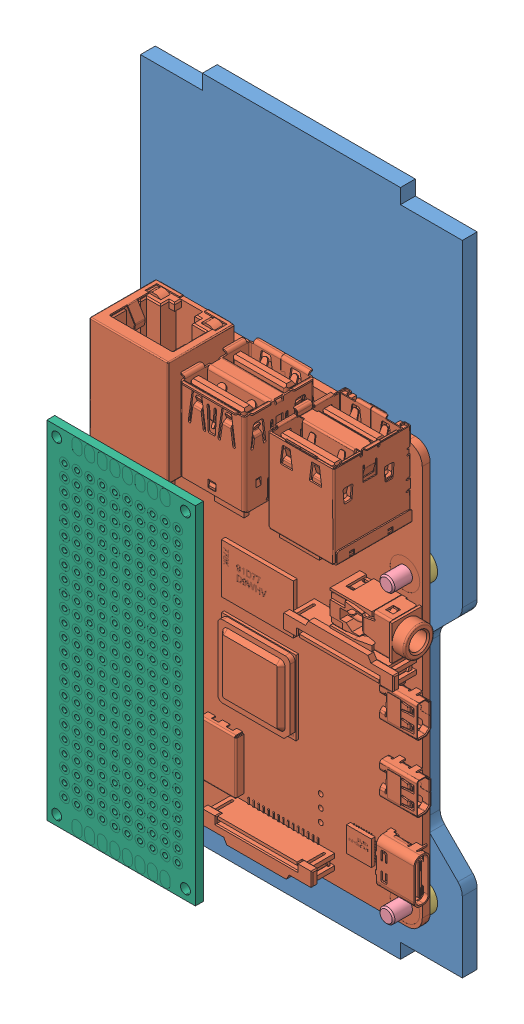
SolidWorks assembly ASM-level-raspberry-pi, configuration По умолчанию. Lengths in mm.
Overall size (65 135 24.74).
13 component instances, 6 part files, 17 mates.
Components (placement in the parent):
- level-2-1: level-2 [По умолчанию] at origin size (65 135 3)
- Raspberry Pi 4 Model B-1: Raspberry Pi 4 Model B [По умолчанию] at (0 -15 5.79) x (0 1 0) z (1 0 0) size (88.99 19.91 58.4)
- 3-6-3-1: 3-6-3 [По умолчанию] at (-24.5 -54 3) size (6 6 2)
- 3-6-3-2: 3-6-3 [По умолчанию] at (-24.5 4 3) size (6 6 2)
- 3-6-3-3: 3-6-3 [По умолчанию] at (24.5 4 3) size (6 6 2)
- 3-6-3-4: 3-6-3 [По умолчанию] at (24.5 -54 3) x (0.98212 -0.188257 0) z (0 0 1) size (6 6 2)
- socket countersunk head screw_iso-1: socket countersunk head screw_iso [ISO 10642 - M3 x 10 - 10N] at (24.5 -54 0.39) x (0 0 1) z (-0.999977 -0.006797 0) size (10 5.54 5.54)
- socket countersunk head screw_iso-2: socket countersunk head screw_iso [ISO 10642 - M3 x 10 - 10N] at (24.5 4 0.39) x (0 0 1) z (-0.999917 -0.012873 0) size (10 5.54 5.54)
- socket countersunk head screw_iso-3: socket countersunk head screw_iso [ISO 10642 - M3 x 10 - 10N] at (-24.5 4 0.39) x (0 0 1) z (-0.999928 -0.012001 0) size (10 5.54 5.54)
- socket countersunk head screw_iso-4: socket countersunk head screw_iso [ISO 10642 - M3 x 10 - 10N] at (-24.5 -54 0.39) x (0 0 1) z (-1 -0.000767 0) size (10 5.54 5.54)
- ASM-shild-raspberry-1: ASM-shild-raspberry [По умолчанию] at (-22.18 0.88 25.14) x (1 0 0) z (0 1 0) size (30 10.65 70)
  - 40 pin connector header smt v3.step-1: 40 pin connector header smt v3.step [По умолчанию] at origin size (5.18 10.05 51.4)
  - Breadboard 30 х 70 mm.step-1: Breadboard 30 х 70 mm.step [По умолчанию] at (7.5097 0.4 -23.0097) size (30 1.65 70)
Mates (geometry in assembly coordinates):
- Концентричный1: concentric anti-aligned: cylinder of level-2-1 through (-24.5 -54 -7) axis (0 0 1) radius 1.75; cylinder of 3-6-3-1 through (-24.5 -54 5) axis (0 0 -1) radius 1.75
- Концентричный2: concentric anti-aligned: cylinder of level-2-1 through (-24.5 4 -7) axis (0 0 1) radius 1.75; cylinder of 3-6-3-2 through (-24.5 4 5) axis (0 0 -1) radius 1.75
- Концентричный3: concentric anti-aligned: cylinder of level-2-1 through (24.5 4 -7) axis (0 0 1) radius 1.75; cylinder of 3-6-3-3 through (24.5 4 5) axis (0 0 -1) radius 1.75
- Концентричный4: concentric anti-aligned: cylinder of level-2-1 through (24.5 -54 -7) axis (0 0 1) radius 1.75; cylinder of 3-6-3-4 through (24.5 -54 5) axis (0 0 -1) radius 1.75
- Совпадение1: coincident aligned: plane of 3-6-3-1 through (-24.5 -54 5) normal (0 0 1); plane of 3-6-3-4 through (24.5 -54 5) normal (0 0 1)
- Совпадение2: coincident aligned: plane of 3-6-3-2 through (-24.5 4 5) normal (0 0 1); plane of 3-6-3-3 through (24.5 4 5) normal (0 0 1)
- Совпадение3: coincident aligned: plane of 3-6-3-3 through (24.5 4 5) normal (0 0 1); plane of 3-6-3-4 through (24.5 -54 5) normal (0 0 1)
- Совпадение4: coincident anti-aligned: plane of level-2-1 through (0 0 3) normal (0 0 1); plane of 3-6-3-4 through (24.5 -54 3) normal (0 0 -1)
- Концентричный5: concentric anti-aligned: cylinder of Raspberry Pi 4 Model B-1 through (24.5 -54 6.59) axis (0 0 1) radius 1.35; cylinder of 3-6-3-4 through (24.5 -54 5) axis (0 0 -1) radius 1.75
- Совпадение5: coincident anti-aligned: plane of Raspberry Pi 4 Model B-1 through (24.5 -54 5) normal (0 0 -1); plane of 3-6-3-4 through (24.5 -54 5) normal (0 0 1)
- Совпадение6: coincident aligned: cone of level-2-1 through (24.5 -54 0) axis (0 0 1); cone of socket countersunk head screw_iso-1 through (24.5 -54 0.98) axis (0 0 1)
- Совпадение7: coincident aligned: cone of level-2-1 through (24.5 4 0) axis (0 0 1); cone of socket countersunk head screw_iso-2 through (24.5 4 0.98) axis (0 0 1)
- Совпадение8: coincident aligned: cone of level-2-1 through (-24.5 4 0) axis (0 0 1); cone of socket countersunk head screw_iso-3 through (-24.5 4 0.98) axis (0 0 1)
- Совпадение9: coincident aligned: cone of level-2-1 through (-24.5 -54 0) axis (0 0 1); cone of socket countersunk head screw_iso-4 through (-24.5 -54 0.98) axis (0 0 1)
- Совпадение10: coincident anti-aligned: plane of Raspberry Pi 4 Model B-1 through (-23.55 -49.45 14.89) normal (0 -1 0); plane of ASM-shild-raspberry-1/40 pin connector header smt v3.step-1 through (-23.91 -49.45 14.09) normal (0 1 0)
- Совпадение11: coincident anti-aligned: plane of Raspberry Pi 4 Model B-1 through (-22.91 -49.45 14.89) normal (1 0 0); plane of ASM-shild-raspberry-1/40 pin connector header smt v3.step-1 through (-22.91 -49.45 14.09) normal (-1 0 0)
- Расстояние1: distance = 5 mm anti-aligned: plane of Raspberry Pi 4 Model B-1 through (-25.77 -49.13 9.09) normal (0 0 1); plane of ASM-shild-raspberry-1/40 pin connector header smt v3.step-1 through (-24.68 -24.82 14.09) normal (0 0 -1)
